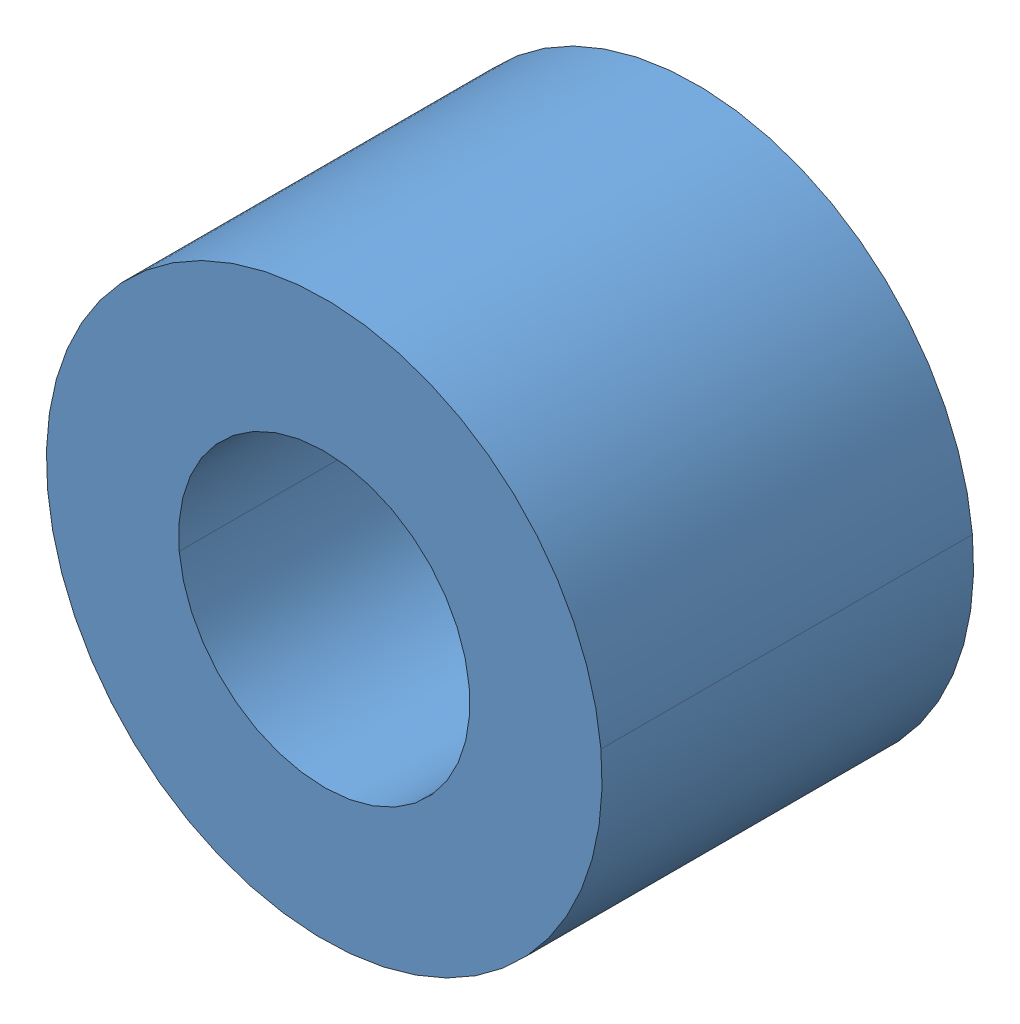
SolidWorks assembly WCP - GreyT Elevator (Cascade, 2 Stage) (1).step, configuration Default. Lengths in mm.
Overall size (10.35 10.35 6.35).
407 component instances, 66 part files, 0 mates.
Components (placement in the parent):
- WCP-0323 - Elevator Clamping Block.step-1: WCP-0323 - Elevator Clamping Block.step [Default] at (152.3365 1149.35 -25.4) x (0 0 1) z (-1 0 0) size (29.22 25.41 49.35) (hidden)
  - WCP-0323-001 Rev2.step-1: WCP-0323-001 Rev2.step [Default] at origin size (20.38 25.41 40.49)
  - WCP-0498 Rev1.step-1: WCP-0498 Rev1.step [Default] at (2.254 0 6.7) x (0 0.307359 0.951594) z (-1 0 0) size (12 12 4)
  - WCP-0212_0_250_radial_bearing.step-1: WCP-0212_0_250_radial_bearing.step [Default] at (-9.525 0 15.4781) size (19.05 19.05 7.14)
  - WCP-0473 Rev1.step-1: WCP-0473 Rev1.step [Default] at (-9.525 0 10.4394) x (-0.082744 -0.996571 0) z (-0.996571 0.082744 0) size (9.53 20.65 9.53)
  - #8-32 x .25L BHCS.step-1: #8-32 x .25L BHCS.step [Default] at (6.7178 0 6.7) x (0 -0.337236 -0.94142) z (1 0 0) size (10.28 8 12.02)
- WCP-0323 - Elevator Clamping Block-1.step-1: WCP-0323 - Elevator Clamping Block-1.step [Default] at (152.3365 1149.35 25.4) x (0 0 -1) z (-1 0 0) size (29.22 25.41 49.35) (hidden)
  - WCP-0323-001 Rev2.step-1: WCP-0323-001 Rev2.step [Default] at origin size (20.38 25.41 40.49)
  - WCP-0498 Rev1.step-1: WCP-0498 Rev1.step [Default] at (2.254 0 6.7) x (0 0.307359 0.951594) z (-1 0 0) size (12 12 4)
  - WCP-0212_0_250_radial_bearing.step-1: WCP-0212_0_250_radial_bearing.step [Default] at (-9.525 0 15.4781) size (19.05 19.05 7.14)
  - WCP-0473 Rev1.step-1: WCP-0473 Rev1.step [Default] at (-9.525 0 10.4394) x (-0.082744 -0.996571 0) z (-0.996571 0.082744 0) size (9.53 20.65 9.53)
  - #8-32 x .25L BHCS.step-1: #8-32 x .25L BHCS.step [Default] at (6.7178 0 6.7) x (0 -0.337236 -0.94142) z (1 0 0) size (10.28 8 12.02)
- WCP-0323 - Elevator Clamping Block-2.step-1: WCP-0323 - Elevator Clamping Block-2.step [Default] at (139.7635 57.15 25.4) x (0 0 -1) z (1 0 0) size (29.22 25.41 49.35) (hidden)
  - WCP-0323-001 Rev2.step-1: WCP-0323-001 Rev2.step [Default] at origin size (20.38 25.41 40.49)
  - WCP-0498 Rev1.step-1: WCP-0498 Rev1.step [Default] at (2.254 0 6.7) x (0 0.307359 0.951594) z (-1 0 0) size (12 12 4)
  - WCP-0212_0_250_radial_bearing.step-1: WCP-0212_0_250_radial_bearing.step [Default] at (-9.525 0 15.4781) size (19.05 19.05 7.14)
  - WCP-0473 Rev1.step-1: WCP-0473 Rev1.step [Default] at (-9.525 0 10.4394) x (-0.082744 -0.996571 0) z (-0.996571 0.082744 0) size (9.53 20.65 9.53)
  - #8-32 x .25L BHCS.step-1: #8-32 x .25L BHCS.step [Default] at (6.7178 0 6.7) x (0 -0.337236 -0.94142) z (1 0 0) size (10.28 8 12.02)
- WCP-0323 - Elevator Clamping Block-3.step-1: WCP-0323 - Elevator Clamping Block-3.step [Default] at (139.7635 57.15 -25.4) x (0 0 1) z (1 0 0) size (29.22 25.41 49.35) (hidden)
  - WCP-0323-001 Rev2.step-1: WCP-0323-001 Rev2.step [Default] at origin size (20.38 25.41 40.49)
  - WCP-0498 Rev1.step-1: WCP-0498 Rev1.step [Default] at (2.254 0 6.7) x (0 0.307359 0.951594) z (-1 0 0) size (12 12 4)
  - WCP-0212_0_250_radial_bearing.step-1: WCP-0212_0_250_radial_bearing.step [Default] at (-9.525 0 15.4781) size (19.05 19.05 7.14)
  - WCP-0473 Rev1.step-1: WCP-0473 Rev1.step [Default] at (-9.525 0 10.4394) x (-0.082744 -0.996571 0) z (-0.996571 0.082744 0) size (9.53 20.65 9.53)
  - #8-32 x .25L BHCS.step-1: #8-32 x .25L BHCS.step [Default] at (6.7178 0 6.7) x (0 -0.337236 -0.94142) z (1 0 0) size (10.28 8 12.02)
- WCP-0323 - Elevator Clamping Block-4.step-1: WCP-0323 - Elevator Clamping Block-4.step [Default] at (101.6635 82.55 25.4) x (0 0 -1) z (1 0 0) size (29.22 25.41 49.35) (hidden)
  - WCP-0323-001 Rev2.step-1: WCP-0323-001 Rev2.step [Default] at origin size (20.38 25.41 40.49)
  - WCP-0498 Rev1.step-1: WCP-0498 Rev1.step [Default] at (2.254 0 6.7) x (0 0.307359 0.951594) z (-1 0 0) size (12 12 4)
  - WCP-0212_0_250_radial_bearing.step-1: WCP-0212_0_250_radial_bearing.step [Default] at (-9.525 0 15.4781) size (19.05 19.05 7.14)
  - WCP-0473 Rev1.step-1: WCP-0473 Rev1.step [Default] at (-9.525 0 10.4394) x (-0.082744 -0.996571 0) z (-0.996571 0.082744 0) size (9.53 20.65 9.53)
  - #8-32 x .25L BHCS.step-1: #8-32 x .25L BHCS.step [Default] at (6.7178 0 6.7) x (0 -0.337236 -0.94142) z (1 0 0) size (10.28 8 12.02)
- WCP-0323 - Elevator Clamping Block-5.step-1: WCP-0323 - Elevator Clamping Block-5.step [Default] at (101.6635 82.55 -25.4) x (0 0 1) z (1 0 0) size (29.22 25.41 49.35) (hidden)
  - WCP-0323-001 Rev2.step-1: WCP-0323-001 Rev2.step [Default] at origin size (20.38 25.41 40.49)
  - WCP-0498 Rev1.step-1: WCP-0498 Rev1.step [Default] at (2.254 0 6.7) x (0 0.307359 0.951594) z (-1 0 0) size (12 12 4)
  - WCP-0212_0_250_radial_bearing.step-1: WCP-0212_0_250_radial_bearing.step [Default] at (-9.525 0 15.4781) size (19.05 19.05 7.14)
  - WCP-0473 Rev1.step-1: WCP-0473 Rev1.step [Default] at (-9.525 0 10.4394) x (-0.082744 -0.996571 0) z (-0.996571 0.082744 0) size (9.53 20.65 9.53)
  - #8-32 x .25L BHCS.step-1: #8-32 x .25L BHCS.step [Default] at (6.7178 0 6.7) x (0 -0.337236 -0.94142) z (1 0 0) size (10.28 8 12.02)
- WCP-0323 - Elevator Clamping Block-6.step-1: WCP-0323 - Elevator Clamping Block-6.step [Default] at (101.6635 222.25 25.4) x (0 0 -1) z (1 0 0) size (29.22 25.41 49.35) (hidden)
  - WCP-0323-001 Rev2.step-1: WCP-0323-001 Rev2.step [Default] at origin size (20.38 25.41 40.49)
  - WCP-0498 Rev1.step-1: WCP-0498 Rev1.step [Default] at (2.254 0 6.7) x (0 0.307359 0.951594) z (-1 0 0) size (12 12 4)
  - WCP-0212_0_250_radial_bearing.step-1: WCP-0212_0_250_radial_bearing.step [Default] at (-9.525 0 15.4781) size (19.05 19.05 7.14)
  - WCP-0473 Rev1.step-1: WCP-0473 Rev1.step [Default] at (-9.525 0 10.4394) x (-0.082744 -0.996571 0) z (-0.996571 0.082744 0) size (9.53 20.65 9.53)
  - #8-32 x .25L BHCS.step-1: #8-32 x .25L BHCS.step [Default] at (6.7178 0 6.7) x (0 -0.337236 -0.94142) z (1 0 0) size (10.28 8 12.02)
- WCP-0323 - Elevator Clamping Block-7.step-1: WCP-0323 - Elevator Clamping Block-7.step [Default] at (101.6635 222.25 -25.4) x (0 0 1) z (1 0 0) size (29.22 25.41 49.35) (hidden)
  - WCP-0323-001 Rev2.step-1: WCP-0323-001 Rev2.step [Default] at origin size (20.38 25.41 40.49)
  - WCP-0498 Rev1.step-1: WCP-0498 Rev1.step [Default] at (2.254 0 6.7) x (0 0.307359 0.951594) z (-1 0 0) size (12 12 4)
  - WCP-0212_0_250_radial_bearing.step-1: WCP-0212_0_250_radial_bearing.step [Default] at (-9.525 0 15.4781) size (19.05 19.05 7.14)
  - WCP-0473 Rev1.step-1: WCP-0473 Rev1.step [Default] at (-9.525 0 10.4394) x (-0.082744 -0.996571 0) z (-0.996571 0.082744 0) size (9.53 20.65 9.53)
  - #8-32 x .25L BHCS.step-1: #8-32 x .25L BHCS.step [Default] at (6.7178 0 6.7) x (0 -0.337236 -0.94142) z (1 0 0) size (10.28 8 12.02)
- WCP-0248 Rev1 - #35 Chain Turnbuckle.step-1: WCP-0248 Rev1 - #35 Chain Turnbuckle.step [Default] at (88.9 1124.7437 -66.675) x (0 -1 0) z (0 0 1) size (55.56 15.05 15.04) (hidden)
  - WCP-0247-001 Rev1.step-1: WCP-0247-001 Rev1.step [Default] at origin size (30.16 9.53 11)
  - NFS-0040_#10-32_jam_nut_left_hand_99961A520.step-1: NFS-0040_#10-32_jam_nut_left_hand_99961A520.step [Default] at (-16.6687 0 0) x (0 0.5 -0.866025) z (0 0.866025 0.5) size (11.01 3.2 11.02)
  - NFS-0037_#10-32_jam_nut_90480A195.step-1: NFS-0037_#10-32_jam_nut_90480A195.step [Default] at (16.6687 0 0) x (0 0.5 0.866025) z (0 -0.866025 0.5) size (11.01 3.2 11.02)
  - WCP-0248-001 Rev1.step-1: WCP-0248-001 Rev1.step [Default] at (23.8125 0 0) x (0 0 1) z (0 1 0) size (9 25.4 9)
  - WCP-0248-002 Rev1.step-1: WCP-0248-002 Rev1.step [Default] at (-23.8125 0 0) x (0 0 -1) z (0 1 0) size (9 25.4 9)
- WCP-0247 Rev1 - #25 Chain Turnbuckle.step-1: WCP-0247 Rev1 - #25 Chain Turnbuckle.step [Default] at (-47.6339 1117.6 -50.8) x (0 1 0) z (-1 0 0) size (50.8 15.05 15.04) (hidden)
  - WCP-0247-001 Rev1.step-1: WCP-0247-001 Rev1.step [Default] at origin size (30.16 9.53 11)
  - NFS-0040_#10-32_jam_nut_left_hand_99961A520.step-1: NFS-0040_#10-32_jam_nut_left_hand_99961A520.step [Default] at (-16.6687 0 0) x (0 0.5 -0.866025) z (0 0.866025 0.5) size (11.01 3.2 11.02)
  - NFS-0037_#10-32_jam_nut_90480A195.step-1: NFS-0037_#10-32_jam_nut_90480A195.step [Default] at (16.6687 0 0) x (0 0.5 0.866025) z (0 -0.866025 0.5) size (11.01 3.2 11.02)
  - WCP-0247-002 Rev2.step-1: WCP-0247-002 Rev2.step [Default] at (22.225 0 0) x (0 0 1) z (0 1 0) size (9 23.02 5.21)
  - WCP-0247-003 Rev2.step-1: WCP-0247-003 Rev2.step [Default] at (-22.225 0 0) x (0 0 -1) z (0 1 0) size (9 23.02 5.21)
- WCP-0323 - Elevator Clamping Block-8.step-1: WCP-0323 - Elevator Clamping Block-8.step [Default] at (-152.3365 1149.35 25.4) x (0 0 -1) z (1 0 0) size (29.22 25.41 49.35) (hidden)
  - WCP-0323-001 Rev2.step-1: WCP-0323-001 Rev2.step [Default] at origin size (20.38 25.41 40.49)
  - WCP-0498 Rev1.step-1: WCP-0498 Rev1.step [Default] at (2.254 0 6.7) x (0 0.307359 0.951594) z (-1 0 0) size (12 12 4)
  - WCP-0212_0_250_radial_bearing.step-1: WCP-0212_0_250_radial_bearing.step [Default] at (-9.525 0 15.4781) size (19.05 19.05 7.14)
  - WCP-0473 Rev1.step-1: WCP-0473 Rev1.step [Default] at (-9.525 0 10.4394) x (-0.082744 -0.996571 0) z (-0.996571 0.082744 0) size (9.53 20.65 9.53)
  - #8-32 x .25L BHCS.step-1: #8-32 x .25L BHCS.step [Default] at (6.7178 0 6.7) x (0 -0.337236 -0.94142) z (1 0 0) size (10.28 8 12.02)
- WCP-0323 - Elevator Clamping Block-9.step-1: WCP-0323 - Elevator Clamping Block-9.step [Default] at (-152.3365 1149.35 -25.4) x (0 0 1) z (1 0 0) size (29.22 25.41 49.35) (hidden)
  - WCP-0323-001 Rev2.step-1: WCP-0323-001 Rev2.step [Default] at origin size (20.38 25.41 40.49)
  - WCP-0498 Rev1.step-1: WCP-0498 Rev1.step [Default] at (2.254 0 6.7) x (0 0.307359 0.951594) z (-1 0 0) size (12 12 4)
  - WCP-0212_0_250_radial_bearing.step-1: WCP-0212_0_250_radial_bearing.step [Default] at (-9.525 0 15.4781) size (19.05 19.05 7.14)
  - WCP-0473 Rev1.step-1: WCP-0473 Rev1.step [Default] at (-9.525 0 10.4394) x (-0.082744 -0.996571 0) z (-0.996571 0.082744 0) size (9.53 20.65 9.53)
  - #8-32 x .25L BHCS.step-1: #8-32 x .25L BHCS.step [Default] at (6.7178 0 6.7) x (0 -0.337236 -0.94142) z (1 0 0) size (10.28 8 12.02)
- WCP-0583 Rev1 - Cascade Pulley Block.step-1: WCP-0583 Rev1 - Cascade Pulley Block.step [Default] at (88.9 25.4 -25.4) x (1 0 0) z (0 1 0) size (47.02 52.05 52.05) (hidden)
  - WCP-0096 Rev6.step-1: WCP-0096 Rev6.step [Default] at (0 25.4 6.35) size (12.65 52.05 52.05)
    - WCP-0096-001 Rev6.step-1: WCP-0096-001 Rev6.step [Default] at origin size (7.57 38.1 38.1)
    - WCP-0096-001 Rev6.step-2: WCP-0096-001 Rev6.step [Default] x (-1 0 0) z (0 0.866025 -0.5) size (7.57 38.1 38.1)
    - WCP-0356 Rev1.step-1: WCP-0356 Rev1.step [Default] at (0.4817 -4.7625 -8.2489) x (0 -0.126969 0.991907) z (0 -0.991907 -0.126969) size (4.06 11.05 4.06)
    - WCP-0356 Rev1.step-2: WCP-0356 Rev1.step [Default] at (0.4817 9.525 0) x (0 0.866766 0.498715) z (0 -0.498715 0.866766) size (4.06 11.05 4.06)
    - WCP-0356 Rev1.step-3: WCP-0356 Rev1.step [Default] at (0.4817 -4.7625 8.2489) x (0 -0.994015 -0.109248) z (0 0.109248 -0.994015) size (4.06 11.05 4.06)
    - WCP-0356 Rev1.step-4: WCP-0356 Rev1.step [Default] at (-0.4817 4.7625 -8.2489) x (0 -0.997555 0.069879) z (0 0.069879 0.997555) size (4.06 11.05 4.06)
    - WCP-0356 Rev1.step-5: WCP-0356 Rev1.step [Default] at (-0.4817 4.7625 8.2489) x (0 -0.7202 -0.693767) z (0 -0.693767 0.7202) size (4.06 11.05 4.06)
    - WCP-0356 Rev1.step-6: WCP-0356 Rev1.step [Default] at (-0.4817 -9.525 0) x (0 -0.997555 0.069879) z (0 0.069879 0.997555) size (4.06 11.05 4.06)
  - WCP-0583-001 Rev1.step-1: WCP-0583-001 Rev1.step [Default] at origin size (34.92 31.75 25.4)
  - WCP-0567 Rev1.step-1: WCP-0567 Rev1.step [Default] at (-6.3246 25.4 6.35) x (0 0 1) z (-1 0 0) size (15.88 15.88 7.94)
  - WCP-0567 Rev1.step-2: WCP-0567 Rev1.step [Default] at (6.3246 25.4 6.35) x (0 0 1) z (1 0 0) size (15.88 15.88 7.94)
  - WCP-0203 Rev1.step-1: WCP-0203 Rev1.step [Default] at (0 25.4 6.35) size (15.88 9.5 9.5)
  - 10-32 BHCS - No Thread_WCP-0258 - 1.750.step-1: 10-32 BHCS - No Thread_WCP-0258 - 1.750.step [Default] at (-17.4625 25.4 6.35) x (0 -0.816967 0.576685) z (0 -0.576685 -0.816967) size (9.17 47.02 9.17)
  - WCP-0326 Rev1.step-1: WCP-0326 Rev1.step [Default] at (19.8374 25.4 6.35) x (0 0.003214 -0.999995) z (0 -0.999995 -0.003214) size (11.02 4.76 11)
- WCP-0583 Rev1 - Cascade Pulley Block-1.step-1: WCP-0583 Rev1 - Cascade Pulley Block-1.step [Default] at (88.9 1219.2 -25.4) x (1 0 0) z (0 1 0) size (47.02 52.05 52.05) (hidden)
  - WCP-0096 Rev6-1.step-1: WCP-0096 Rev6-1.step [Default] at (0 25.4 6.35) size (12.65 52.05 52.05)
    - WCP-0096-001 Rev6.step-1: WCP-0096-001 Rev6.step [Default] at origin size (7.57 38.1 38.1)
    - WCP-0096-001 Rev6.step-2: WCP-0096-001 Rev6.step [Default] x (-1 0 0) z (0 0.866025 -0.5) size (7.57 38.1 38.1)
    - WCP-0356 Rev1.step-1: WCP-0356 Rev1.step [Default] at (0.4817 -4.7625 -8.2489) x (0 -0.126969 0.991907) z (0 -0.991907 -0.126969) size (4.06 11.05 4.06)
    - WCP-0356 Rev1.step-2: WCP-0356 Rev1.step [Default] at (0.4817 9.525 0) x (0 0.866766 0.498715) z (0 -0.498715 0.866766) size (4.06 11.05 4.06)
    - WCP-0356 Rev1.step-3: WCP-0356 Rev1.step [Default] at (0.4817 -4.7625 8.2489) x (0 -0.994015 -0.109248) z (0 0.109248 -0.994015) size (4.06 11.05 4.06)
    - WCP-0356 Rev1.step-4: WCP-0356 Rev1.step [Default] at (-0.4817 4.7625 -8.2489) x (0 -0.997555 0.069879) z (0 0.069879 0.997555) size (4.06 11.05 4.06)
    - WCP-0356 Rev1.step-5: WCP-0356 Rev1.step [Default] at (-0.4817 4.7625 8.2489) x (0 -0.7202 -0.693767) z (0 -0.693767 0.7202) size (4.06 11.05 4.06)
    - WCP-0356 Rev1.step-6: WCP-0356 Rev1.step [Default] at (-0.4817 -9.525 0) x (0 -0.997555 0.069879) z (0 0.069879 0.997555) size (4.06 11.05 4.06)
  - WCP-0583-001 Rev1.step-1: WCP-0583-001 Rev1.step [Default] at origin size (34.92 31.75 25.4)
  - WCP-0567 Rev1.step-1: WCP-0567 Rev1.step [Default] at (-6.3246 25.4 6.35) x (0 0 1) z (-1 0 0) size (15.88 15.88 7.94)
  - WCP-0567 Rev1.step-2: WCP-0567 Rev1.step [Default] at (6.3246 25.4 6.35) x (0 0 1) z (1 0 0) size (15.88 15.88 7.94)
  - WCP-0203 Rev1.step-1: WCP-0203 Rev1.step [Default] at (0 25.4 6.35) size (15.88 9.5 9.5)
  - 10-32 BHCS - No Thread_WCP-0258 - 1.750.step-1: 10-32 BHCS - No Thread_WCP-0258 - 1.750.step [Default] at (-17.4625 25.4 6.35) x (0 -0.816967 0.576685) z (0 -0.576685 -0.816967) size (9.17 47.02 9.17)
  - WCP-0326 Rev1.step-1: WCP-0326 Rev1.step [Default] at (19.8374 25.4 6.35) x (0 0.003214 -0.999995) z (0 -0.999995 -0.003214) size (11.02 4.76 11)
- WCP-0583 Rev1 - Cascade Pulley Block_Mirrored.step-1: WCP-0583 Rev1 - Cascade Pulley Block_Mirrored.step [Default] at (-88.9 1219.2 -25.4) x (1 0 0) z (0 1 0) size (47.02 52.05 52.05) (hidden)
  - WCP-0096 Rev6-2.step-1: WCP-0096 Rev6-2.step [Default] at (0 25.4 6.35) size (12.65 52.05 52.05)
    - WCP-0096-001 Rev6.step-1: WCP-0096-001 Rev6.step [Default] at origin size (7.57 38.1 38.1)
    - WCP-0096-001 Rev6.step-2: WCP-0096-001 Rev6.step [Default] x (-1 0 0) z (0 0.866025 -0.5) size (7.57 38.1 38.1)
    - WCP-0356 Rev1.step-1: WCP-0356 Rev1.step [Default] at (0.4817 -4.7625 -8.2489) x (0 -0.126969 0.991907) z (0 -0.991907 -0.126969) size (4.06 11.05 4.06)
    - WCP-0356 Rev1.step-2: WCP-0356 Rev1.step [Default] at (0.4817 9.525 0) x (0 0.866766 0.498715) z (0 -0.498715 0.866766) size (4.06 11.05 4.06)
    - WCP-0356 Rev1.step-3: WCP-0356 Rev1.step [Default] at (0.4817 -4.7625 8.2489) x (0 -0.994015 -0.109248) z (0 0.109248 -0.994015) size (4.06 11.05 4.06)
    - WCP-0356 Rev1.step-4: WCP-0356 Rev1.step [Default] at (-0.4817 4.7625 -8.2489) x (0 -0.997555 0.069879) z (0 0.069879 0.997555) size (4.06 11.05 4.06)
    - WCP-0356 Rev1.step-5: WCP-0356 Rev1.step [Default] at (-0.4817 4.7625 8.2489) x (0 -0.7202 -0.693767) z (0 -0.693767 0.7202) size (4.06 11.05 4.06)
    - WCP-0356 Rev1.step-6: WCP-0356 Rev1.step [Default] at (-0.4817 -9.525 0) x (0 -0.997555 0.069879) z (0 0.069879 0.997555) size (4.06 11.05 4.06)
  - WCP-0583-001 Rev1.step-1: WCP-0583-001 Rev1.step [Default] at origin size (34.92 31.75 25.4)
  - WCP-0567 Rev1.step-1: WCP-0567 Rev1.step [Default] at (-6.3246 25.4 6.35) x (0 0 1) z (-1 0 0) size (15.88 15.88 7.94)
  - WCP-0567 Rev1.step-2: WCP-0567 Rev1.step [Default] at (6.3246 25.4 6.35) x (0 0 1) z (1 0 0) size (15.88 15.88 7.94)
  - WCP-0203 Rev1.step-1: WCP-0203 Rev1.step [Default] at (0 25.4 6.35) size (15.88 9.5 9.5)
  - 10-32 BHCS - No Thread_WCP-0258 - 1.750.step-1: 10-32 BHCS - No Thread_WCP-0258 - 1.750.step [Default] at (17.4625 25.4 6.35) x (0 0.844944 -0.534854) z (0 -0.534854 -0.844944) size (9.17 47.02 9.17)
  - WCP-0326 Rev1.step-1: WCP-0326 Rev1.step [Default] at (-19.8374 25.4 6.35) x (0 -0.925447 -0.378877) z (0 0.378877 -0.925447) size (11.02 4.76 11)
- WCP-0583 Rev1 - Cascade Pulley Block_Mirrored-1.step-1: WCP-0583 Rev1 - Cascade Pulley Block_Mirrored-1.step [Default] at (-88.9 25.4 -25.4) x (1 0 0) z (0 1 0) size (47.02 52.05 52.05) (hidden)
  - WCP-0096 Rev6-3.step-1: WCP-0096 Rev6-3.step [Default] at (0 25.4 6.35) size (12.65 52.05 52.05)
    - WCP-0096-001 Rev6.step-1: WCP-0096-001 Rev6.step [Default] at origin size (7.57 38.1 38.1)
    - WCP-0096-001 Rev6.step-2: WCP-0096-001 Rev6.step [Default] x (-1 0 0) z (0 0.866025 -0.5) size (7.57 38.1 38.1)
    - WCP-0356 Rev1.step-1: WCP-0356 Rev1.step [Default] at (0.4817 -4.7625 -8.2489) x (0 -0.126969 0.991907) z (0 -0.991907 -0.126969) size (4.06 11.05 4.06)
    - WCP-0356 Rev1.step-2: WCP-0356 Rev1.step [Default] at (0.4817 9.525 0) x (0 0.866766 0.498715) z (0 -0.498715 0.866766) size (4.06 11.05 4.06)
    - WCP-0356 Rev1.step-3: WCP-0356 Rev1.step [Default] at (0.4817 -4.7625 8.2489) x (0 -0.994015 -0.109248) z (0 0.109248 -0.994015) size (4.06 11.05 4.06)
    - WCP-0356 Rev1.step-4: WCP-0356 Rev1.step [Default] at (-0.4817 4.7625 -8.2489) x (0 -0.997555 0.069879) z (0 0.069879 0.997555) size (4.06 11.05 4.06)
    - WCP-0356 Rev1.step-5: WCP-0356 Rev1.step [Default] at (-0.4817 4.7625 8.2489) x (0 -0.7202 -0.693767) z (0 -0.693767 0.7202) size (4.06 11.05 4.06)
    - WCP-0356 Rev1.step-6: WCP-0356 Rev1.step [Default] at (-0.4817 -9.525 0) x (0 -0.997555 0.069879) z (0 0.069879 0.997555) size (4.06 11.05 4.06)
  - WCP-0583-001 Rev1.step-1: WCP-0583-001 Rev1.step [Default] at origin size (34.92 31.75 25.4)
  - WCP-0567 Rev1.step-1: WCP-0567 Rev1.step [Default] at (-6.3246 25.4 6.35) x (0 0 1) z (-1 0 0) size (15.88 15.88 7.94)
  - WCP-0567 Rev1.step-2: WCP-0567 Rev1.step [Default] at (6.3246 25.4 6.35) x (0 0 1) z (1 0 0) size (15.88 15.88 7.94)
  - WCP-0203 Rev1.step-1: WCP-0203 Rev1.step [Default] at (0 25.4 6.35) size (15.88 9.5 9.5)
  - 10-32 BHCS - No Thread_WCP-0258 - 1.750.step-1: 10-32 BHCS - No Thread_WCP-0258 - 1.750.step [Default] at (17.4625 25.4 6.35) x (0 0.844944 -0.534854) z (0 -0.534854 -0.844944) size (9.17 47.02 9.17)
  - WCP-0326 Rev1.step-1: WCP-0326 Rev1.step [Default] at (-19.8374 25.4 6.35) x (0 -0.925447 -0.378877) z (0 0.378877 -0.925447) size (11.02 4.76 11)
- WCP-0323 - Elevator Clamping Block-10.step-1: WCP-0323 - Elevator Clamping Block-10.step [Default] at (-139.7635 57.15 -25.4) x (0 0 1) z (-1 0 0) size (29.22 25.41 49.35) (hidden)
  - WCP-0323-001 Rev2.step-1: WCP-0323-001 Rev2.step [Default] at origin size (20.38 25.41 40.49)
  - WCP-0498 Rev1.step-1: WCP-0498 Rev1.step [Default] at (2.254 0 6.7) x (0 0.307359 0.951594) z (-1 0 0) size (12 12 4)
  - WCP-0212_0_250_radial_bearing.step-1: WCP-0212_0_250_radial_bearing.step [Default] at (-9.525 0 15.4781) size (19.05 19.05 7.14)
  - WCP-0473 Rev1.step-1: WCP-0473 Rev1.step [Default] at (-9.525 0 10.4394) x (-0.082744 -0.996571 0) z (-0.996571 0.082744 0) size (9.53 20.65 9.53)
  - #8-32 x .25L BHCS.step-1: #8-32 x .25L BHCS.step [Default] at (6.7178 0 6.7) x (0 -0.337236 -0.94142) z (1 0 0) size (10.28 8 12.02)
- WCP-0557 Rev1 - WCP Single Stage Gearbox_0.5_ Hex.step-1: WCP-0557 Rev1 - WCP Single Stage Gearbox_0.5_ Hex.step [Default] at (-25.4 0 66.675) x (-1 0 0) z (0 0 -1) size (173.55 82.41 254.05) (hidden)
  - WCP-0557-001 Rev1.step-1: WCP-0557-001 Rev1.step [Default] at origin size (151.92 76.2 6.35)
  - WCP-0557-002 Rev1.step-1: WCP-0557-002 Rev1.step [Default] at (0 0 34.925) size (76.2 76.2 6.35)
  - 217-6515_Falcon_500_Default_As Machined_.step-1: 217-6515_Falcon_500_Default_As Machined_.step [Default] at (45.7962 0 -29.375) x (0.866025 0.5 0) z (0 0 1) size (60 60 115.81)
  - 217-6515_Falcon_500_Default_As Machined_.step-2: 217-6515_Falcon_500_Default_As Machined_.step [Default] at (-45.7962 0 -29.375) x (0.866025 0.5 0) z (0 0 1) size (60 60 115.81)
  - 217-6919_Falcon_12T.step-1: 217-6919_Falcon_12T.step [Default] at (45.7962 0 12.5775) x (0.990666 -0.136309 0) z (0 0 1) size (17.78 17.78 19.05)
  - 217-6919_Falcon_12T.step-2: 217-6919_Falcon_12T.step [Default] at (-45.7962 0 12.5775) x (0.990666 -0.136309 0) z (0 0 1) size (17.78 17.78 19.05)
  - WCP-0226 Rev1.step-1: WCP-0226 Rev1.step [Default] at (32.5438 -32.5438 17.4625) x (0 0 -1) z (0.876265 0.481829 0) size (28.57 9.5 9.5)
  - WCP-0226 Rev1.step-2: WCP-0226 Rev1.step [Default] at (32.5438 32.5438 17.4625) x (0 0 -1) z (-0.524135 0.851635 0) size (28.57 9.5 9.5)
  - WCP-0226 Rev1.step-3: WCP-0226 Rev1.step [Default] at (-32.5438 -32.5438 17.4625) x (0 0 -1) z (0.876265 0.481829 0) size (28.57 9.5 9.5)
  - WCP-0226 Rev1.step-4: WCP-0226 Rev1.step [Default] at (-32.5438 32.5438 17.4625) x (0 0 -1) z (0.876265 0.481829 0) size (28.57 9.5 9.5)
  - WCP-0557-004 Rev1.step-1: WCP-0557-004 Rev1.step [Default] at (0 0 0.7937) x (1 0 0) z (0 -1 0) size (45 7.94 45)
  - WCP-0781_0_500_flanged_bearing.step-1: WCP-0781_0_500_flanged_bearing.step [Default] at (0 0 -3.175) x (0.999832 0.018325 0) z (0.018325 -0.999832 0) size (31.12 7.94 31.12)
  - WCP-0557-004 Rev1.step-2: WCP-0557-004 Rev1.step [Default] at (0 0 34.1313) x (1 0 0) z (0 1 0) size (45 7.94 45)
  - WCP-0790_500L_500_hex.step-1: WCP-0790_500L_500_hex.step [Default] at (0 0 23.7617) x (0.953738 0.300639 0) z (0 0 1) size (19.5 19.5 12.7)
  - 10-32 BHCS - No Thread_WCP-0257 - 1.500.step-1: 10-32 BHCS - No Thread_WCP-0257 - 1.500.step [Default] at (32.5438 32.5438 0) x (0.63562 -0.772002 0) z (0.772002 0.63562 0) size (9.17 40.67 9.17)
  - 10-32 BHCS - No Thread_WCP-0257 - 1.500.step-2: 10-32 BHCS - No Thread_WCP-0257 - 1.500.step [Default] at (-32.5438 32.5438 0) x (0.63562 -0.772002 0) z (0.772002 0.63562 0) size (9.17 40.67 9.17)
  - 10-32 BHCS - No Thread_WCP-0257 - 1.500.step-3: 10-32 BHCS - No Thread_WCP-0257 - 1.500.step [Default] at (32.5438 -32.5438 0) x (0.63562 -0.772002 0) z (0.772002 0.63562 0) size (9.17 40.67 9.17)
  - 10-32 BHCS - No Thread_WCP-0257 - 1.500.step-4: 10-32 BHCS - No Thread_WCP-0257 - 1.500.step [Default] at (-32.5438 -32.5438 0) x (0.63562 -0.772002 0) z (0.772002 0.63562 0) size (9.17 40.67 9.17)
  - 10-32 BHCS - No Thread_WCP-0253 - 0.500.step-1: 10-32 BHCS - No Thread_WCP-0253 - 0.500.step [Default] at (45.7962 25.4 3.175) x (0.313732 -0.949511 0) z (-0.949511 -0.313732 0) size (9.17 15.27 9.17)
  - 10-32 BHCS - No Thread_WCP-0253 - 0.500.step-2: 10-32 BHCS - No Thread_WCP-0253 - 0.500.step [Default] at (45.7962 -25.4 3.175) x (0.270491 -0.962723 0) z (-0.962723 -0.270491 0) size (9.17 15.27 9.17)
  - 10-32 BHCS - No Thread_WCP-0253 - 0.500.step-3: 10-32 BHCS - No Thread_WCP-0253 - 0.500.step [Default] at (-45.7962 25.4 3.175) x (0.363225 -0.931702 0) z (-0.931702 -0.363225 0) size (9.17 15.27 9.17)
  - 10-32 BHCS - No Thread_WCP-0253 - 0.500.step-4: 10-32 BHCS - No Thread_WCP-0253 - 0.500.step [Default] at (-45.7962 -25.4 3.175) x (0.510832 -0.85968 0) z (-0.85968 -0.510832 0) size (9.17 15.27 9.17)
  - WCP-0832 Rev1.step-1: WCP-0832 Rev1.step [Default] at (0 0 87.3125) x (0.457904 0.889002 0) z (0 0 1) size (13.75 13.61 175.64)
  - WCP-0785_0_500_flanged_thunderhex_bearing.step-1: WCP-0785_0_500_flanged_thunderhex_bearing.step [Default] at (0 0 34.1313) x (-0.110978 -0.993823 0) z (0 0 -1) size (31.12 31.12 7.94)
  - WCP-0229 Rev1.step-1: WCP-0229 Rev1.step [Default] at (0 0 -3.6195) x (0 0 1) z (-0.791548 -0.611107 0) size (0.89 16.1 14.34)
  - WCP-0187 Rev1.step-1: WCP-0187 Rev1.step [Default] at (0 0 11.0871) x (0.99882 0.048566 0) z (0 0 1) size (78.68 78.68 12.65)
- WCP-0323 - Elevator Clamping Block-11.step-1: WCP-0323 - Elevator Clamping Block-11.step [Default] at (-101.6635 82.55 -25.4) x (0 0 1) z (-1 0 0) size (29.22 25.41 49.35) (hidden)
  - WCP-0323-001 Rev2.step-1: WCP-0323-001 Rev2.step [Default] at origin size (20.38 25.41 40.49)
  - WCP-0498 Rev1.step-1: WCP-0498 Rev1.step [Default] at (2.254 0 6.7) x (0 0.307359 0.951594) z (-1 0 0) size (12 12 4)
  - WCP-0212_0_250_radial_bearing.step-1: WCP-0212_0_250_radial_bearing.step [Default] at (-9.525 0 15.4781) size (19.05 19.05 7.14)
  - WCP-0473 Rev1.step-1: WCP-0473 Rev1.step [Default] at (-9.525 0 10.4394) x (-0.082744 -0.996571 0) z (-0.996571 0.082744 0) size (9.53 20.65 9.53)
  - #8-32 x .25L BHCS.step-1: #8-32 x .25L BHCS.step [Default] at (6.7178 0 6.7) x (0 -0.337236 -0.94142) z (1 0 0) size (10.28 8 12.02)
- WCP-0323 - Elevator Clamping Block-12.step-1: WCP-0323 - Elevator Clamping Block-12.step [Default] at (-101.6635 82.55 25.4) x (0 0 -1) z (-1 0 0) size (29.22 25.41 49.35) (hidden)
  - WCP-0323-001 Rev2.step-1: WCP-0323-001 Rev2.step [Default] at origin size (20.38 25.41 40.49)
  - WCP-0498 Rev1.step-1: WCP-0498 Rev1.step [Default] at (2.254 0 6.7) x (0 0.307359 0.951594) z (-1 0 0) size (12 12 4)
  - WCP-0212_0_250_radial_bearing.step-1: WCP-0212_0_250_radial_bearing.step [Default] at (-9.525 0 15.4781) size (19.05 19.05 7.14)
  - WCP-0473 Rev1.step-1: WCP-0473 Rev1.step [Default] at (-9.525 0 10.4394) x (-0.082744 -0.996571 0) z (-0.996571 0.082744 0) size (9.53 20.65 9.53)
  - #8-32 x .25L BHCS.step-1: #8-32 x .25L BHCS.step [Default] at (6.7178 0 6.7) x (0 -0.337236 -0.94142) z (1 0 0) size (10.28 8 12.02)
- WCP-0323 - Elevator Clamping Block-13.step-1: WCP-0323 - Elevator Clamping Block-13.step [Default] at (-139.7635 57.15 25.4) x (0 0 -1) z (-1 0 0) size (29.22 25.41 49.35) (hidden)
  - WCP-0323-001 Rev2.step-1: WCP-0323-001 Rev2.step [Default] at origin size (20.38 25.41 40.49)
  - WCP-0498 Rev1.step-1: WCP-0498 Rev1.step [Default] at (2.254 0 6.7) x (0 0.307359 0.951594) z (-1 0 0) size (12 12 4)
  - WCP-0212_0_250_radial_bearing.step-1: WCP-0212_0_250_radial_bearing.step [Default] at (-9.525 0 15.4781) size (19.05 19.05 7.14)
  - WCP-0473 Rev1.step-1: WCP-0473 Rev1.step [Default] at (-9.525 0 10.4394) x (-0.082744 -0.996571 0) z (-0.996571 0.082744 0) size (9.53 20.65 9.53)
  - #8-32 x .25L BHCS.step-1: #8-32 x .25L BHCS.step [Default] at (6.7178 0 6.7) x (0 -0.337236 -0.94142) z (1 0 0) size (10.28 8 12.02)
- WCP-0323 - Elevator Clamping Block-14.step-1: WCP-0323 - Elevator Clamping Block-14.step [Default] at (-101.6635 222.25 -25.4) x (0 0 1) z (-1 0 0) size (29.22 25.41 49.35) (hidden)
  - WCP-0323-001 Rev2.step-1: WCP-0323-001 Rev2.step [Default] at origin size (20.38 25.41 40.49)
  - WCP-0498 Rev1.step-1: WCP-0498 Rev1.step [Default] at (2.254 0 6.7) x (0 0.307359 0.951594) z (-1 0 0) size (12 12 4)
  - WCP-0212_0_250_radial_bearing.step-1: WCP-0212_0_250_radial_bearing.step [Default] at (-9.525 0 15.4781) size (19.05 19.05 7.14)
  - WCP-0473 Rev1.step-1: WCP-0473 Rev1.step [Default] at (-9.525 0 10.4394) x (-0.082744 -0.996571 0) z (-0.996571 0.082744 0) size (9.53 20.65 9.53)
  - #8-32 x .25L BHCS.step-1: #8-32 x .25L BHCS.step [Default] at (6.7178 0 6.7) x (0 -0.337236 -0.94142) z (1 0 0) size (10.28 8 12.02)
- WCP-0323 - Elevator Clamping Block-15.step-1: WCP-0323 - Elevator Clamping Block-15.step [Default] at (-101.6635 222.25 25.4) x (0 0 -1) z (-1 0 0) size (29.22 25.41 49.35) (hidden)
  - WCP-0323-001 Rev2.step-1: WCP-0323-001 Rev2.step [Default] at origin size (20.38 25.41 40.49)
  - WCP-0498 Rev1.step-1: WCP-0498 Rev1.step [Default] at (2.254 0 6.7) x (0 0.307359 0.951594) z (-1 0 0) size (12 12 4)
  - WCP-0212_0_250_radial_bearing.step-1: WCP-0212_0_250_radial_bearing.step [Default] at (-9.525 0 15.4781) size (19.05 19.05 7.14)
  - WCP-0473 Rev1.step-1: WCP-0473 Rev1.step [Default] at (-9.525 0 10.4394) x (-0.082744 -0.996571 0) z (-0.996571 0.082744 0) size (9.53 20.65 9.53)
  - #8-32 x .25L BHCS.step-1: #8-32 x .25L BHCS.step [Default] at (6.7178 0 6.7) x (0 -0.337236 -0.94142) z (1 0 0) size (10.28 8 12.02)
- WCP-0248 Rev1 - #35 Chain Turnbuckle-1.step-1: WCP-0248 Rev1 - #35 Chain Turnbuckle-1.step [Default] at (-88.9 1124.7437 -66.675) x (0 -1 0) z (0 0 -1) size (55.56 15.05 15.04) (hidden)
  - WCP-0247-001 Rev1.step-1: WCP-0247-001 Rev1.step [Default] at origin size (30.16 9.53 11)
  - NFS-0040_#10-32_jam_nut_left_hand_99961A520.step-1: NFS-0040_#10-32_jam_nut_left_hand_99961A520.step [Default] at (-16.6687 0 0) x (0 0.5 -0.866025) z (0 0.866025 0.5) size (11.01 3.2 11.02)
  - NFS-0037_#10-32_jam_nut_90480A195.step-1: NFS-0037_#10-32_jam_nut_90480A195.step [Default] at (16.6687 0 0) x (0 0.5 0.866025) z (0 -0.866025 0.5) size (11.01 3.2 11.02)
  - WCP-0248-001 Rev1.step-1: WCP-0248-001 Rev1.step [Default] at (23.8125 0 0) x (0 0 1) z (0 1 0) size (9 25.4 9)
  - WCP-0248-002 Rev1.step-1: WCP-0248-002 Rev1.step [Default] at (-23.8125 0 0) x (0 0 -1) z (0 1 0) size (9 25.4 9)
- WCP-EX-0019-001.step-1: WCP-EX-0019-001.step [Default] x (1 0 0) z (0 -1 0) size (457.2 50.8 25.4) (hidden)
- WCP-EX-0019-003.step-1: WCP-EX-0019-003.step [Default] at (165.1 609.6 0) x (0 -1 0) z (1 0 0) size (1193.8 50.8 25.4) (hidden)
- WCP-EX-0019-002.step-1: WCP-EX-0019-002.step [Default] at (0 1181.1 -88.9) size (355.6 50.8 25.4) (hidden)
- WCP-EX-0019-004.step-1: WCP-EX-0019-004.step [Default] at (127 622.3 0) x (0 -1 0) z (-1 0 0) size (1219.2 50.8 25.4) (hidden)
- WCP-EX-0019-007.step-1: WCP-EX-0019-007.step [Default] at (0 25.4 0) x (1 0 0) z (0 -1 0) size (228.6 50.8 25.4) (hidden)
- WCP-EX-0019-007.step-2: WCP-EX-0019-007.step [Default] at (0 1219.2 0) x (1 0 0) z (0 -1 0) size (228.6 50.8 25.4) (hidden)
- WCP-EX-0019-005.step-1: WCP-EX-0019-005.step [Default] at (88.9 152.4 0) x (0 -1 0) z (-1 0 0) size (228.6 50.8 25.4) (hidden)
- WCP-EX-0019-006.step-1: WCP-EX-0019-006.step [Default] at (0 50.8 0) x (1 0 0) z (0 -1 0) size (152.4 50.8 25.4) (hidden)
- WCP-EX-0019-006.step-2: WCP-EX-0019-006.step [Default] at (0 254 0) x (1 0 0) z (0 -1 0) size (152.4 50.8 25.4) (hidden)
- WCP-EX-0019-003.step-2: WCP-EX-0019-003.step [Default] at (-165.1 609.6 0) x (0 -1 0) z (1 0 0) size (1193.8 50.8 25.4) (hidden)
- 10-32 BHCS - No Thread_WCP-0261 - 2.500.step-1: 10-32 BHCS - No Thread_WCP-0261 - 2.500.step [Default] at (165.1 1143 30.1625) x (0.999937 0.011255 0) z (0.011255 -0.999937 0) size (9.17 66.07 9.17) (hidden)
- 10-32 BHCS - No Thread_WCP-0261 - 2.500.step-2: 10-32 BHCS - No Thread_WCP-0261 - 2.500.step [Default] at (165.1 1155.7 -30.1625) x (-0.802481 0.596678 0) z (-0.596678 -0.802481 0) size (9.17 66.07 9.17) (hidden)
- 10-32 BHCS - No Thread_WCP-0261 - 2.500.step-3: 10-32 BHCS - No Thread_WCP-0261 - 2.500.step [Default] at (127 50.8 -30.1625) x (-0.742242 0.670132 0) z (-0.670132 -0.742242 0) size (9.17 66.07 9.17) (hidden)
- 10-32 BHCS - No Thread_WCP-0261 - 2.500.step-4: 10-32 BHCS - No Thread_WCP-0261 - 2.500.step [Default] at (127 63.5 30.1625) x (0.985295 -0.170861 0) z (-0.170861 -0.985295 0) size (9.17 66.07 9.17) (hidden)
- 10-32 BHCS - No Thread_WCP-0261 - 2.500.step-5: 10-32 BHCS - No Thread_WCP-0261 - 2.500.step [Default] at (88.9 76.2 -30.1625) x (-0.742242 0.670132 0) z (-0.670132 -0.742242 0) size (9.17 66.07 9.17) (hidden)
- 10-32 BHCS - No Thread_WCP-0261 - 2.500.step-6: 10-32 BHCS - No Thread_WCP-0261 - 2.500.step [Default] at (88.9 88.9 30.1625) x (0.985295 -0.170861 0) z (-0.170861 -0.985295 0) size (9.17 66.07 9.17) (hidden)
- 10-32 BHCS - No Thread_WCP-0261 - 2.500.step-7: 10-32 BHCS - No Thread_WCP-0261 - 2.500.step [Default] at (88.9 215.9 -30.1625) x (-0.742242 0.670132 0) z (-0.670132 -0.742242 0) size (9.17 66.07 9.17) (hidden)
- 10-32 BHCS - No Thread_WCP-0261 - 2.500.step-8: 10-32 BHCS - No Thread_WCP-0261 - 2.500.step [Default] at (88.9 228.6 30.1625) x (0.985295 -0.170861 0) z (-0.170861 -0.985295 0) size (9.17 66.07 9.17) (hidden)
- 10-32 SHCS - No Thread_WCP-0274 - 4.500.step-1: 10-32 SHCS - No Thread_WCP-0274 - 4.500.step [Default] at (165.1 1168.4 -77.7875) x (0.495006 -0.86889 0) z (0.86889 0.495006 0) size (7.67 119.13 7.67) (hidden)
- 10-32 SHCS - No Thread_WCP-0274 - 4.500.step-2: 10-32 SHCS - No Thread_WCP-0274 - 4.500.step [Default] at (165.1 1193.8 -77.7875) x (0.495006 -0.86889 0) z (0.86889 0.495006 0) size (7.67 119.13 7.67) (hidden)
